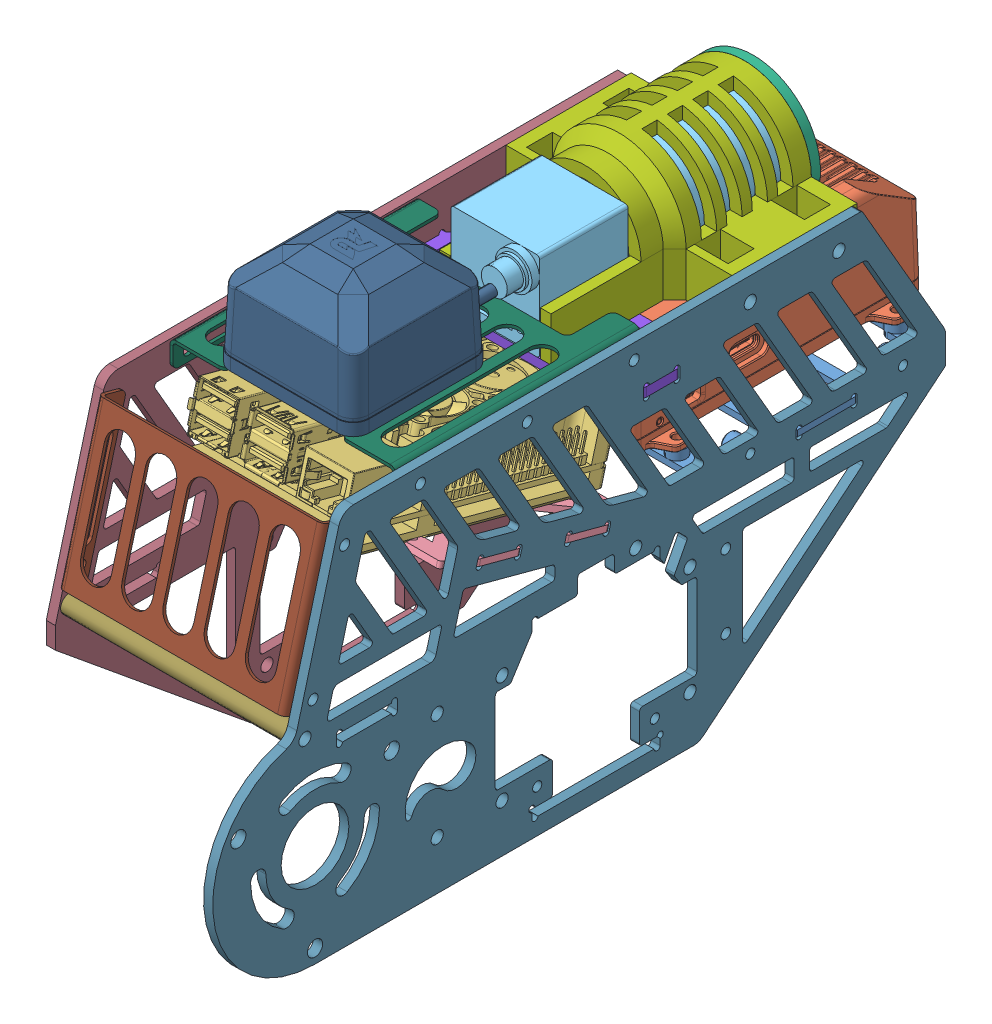
SolidWorks assembly pitch轴顶部设备, configuration 默认. Lengths in mm.
Overall size (80.14 158 249.05).
17 component instances, 15 part files, 47 mates.
Components (placement in the parent):
- 图传安装架-1: 图传安装架 [默认] at origin size (80 6 78)
- RM2019图传模块VT02-1: RM2019图传模块VT02 [默认] at (0 5 0.35) size (60 36.09 100.47)
- Raspberry Pi 4 Model B-1: Raspberry Pi 4 Model B [默认] at (0 22.2544 100.0052) x (0 0.258819 0.965926) z (-1 0 0) size (93.45 25.9 58.4)
- 树莓派安装板-1: 树莓派安装板 [默认] at (0 9.8234 92.9833) x (1 0 0) z (0 0.258819 0.965926) size (80 2 64)
- 相机MER-139-210U3C;HN-0612-2M-C1÷2X-1: 相机MER-139-210U3C;HN-0612-2M-C1÷2X [默认] at (0 53.5 39.5) x (0 1 0) z (1 0 0) size (32.45 89.5 29.5)
- 相机顶部保护PC板-1: 相机顶部保护PC板 [默认] at (0 53.5 -13) x (-1 0 0) z (0 0 -1) size (44 38.5 3)
- 相机顶部保护壳-1: 相机顶部保护壳 [默认] at (0 53.5 39) x (1 0 0) z (0 0 -1) size (74 36.5 81.5)
- 相机顶部安装板-1: 相机顶部安装板 [默认] at (0 36 39.5) size (80 3 29)
- hexagon socket head cap screws gb-1: hexagon socket head cap screws gb [GB_FASTENER_SCREWS_HSHCS M3X6-C] at (-10 33 41.8) x (0 1 0) z (0 0 -1) size (9 5.5 5.5)
- hexagon socket head cap screws gb-3: hexagon socket head cap screws gb [GB_FASTENER_SCREWS_HSHCS M3X6-C] at (10 33 41.8) x (0 1 0) z (0 0 -1) size (9 5.5 5.5)
- RM2019裁判系统定位模块UW01-1: RM2019裁判系统定位模块UW01 [默认] at (0 54 115) x (-1 0 0) z (0 0 -1) size (45.56 33.5 81.86)
- 后端钣金支撑-1: 后端钣金支撑 [默认] at (0 25.3462 167.3322) x (1 0 0) z (0 0.965926 -0.258819) size (74 9 50)
- 铝柱M4×74-定制-1: 铝柱M4×74-定制 [默认] at (37 -5 62.5) x (0 0 1) z (-1 0 0) size (6 6 74)
- 铝柱M4×74-定制-2: 铝柱M4×74-定制 [默认] at (37 -5 170.8047) x (0 0.986463 -0.163981) z (-1 0 0) size (6 6 74)
- pitch轴外框竖板-1: pitch轴外框竖板 [默认] at (-37 -37 75.5) x (-1 0 0) z (0 0 -1) size (3 124 214.5)
- pitch轴外框竖板-电机-1: pitch轴外框竖板-电机 [默认] at (40 -37 75.5) x (-1 0 0) z (0 0 -1) size (3.14 124 240)
- 顶部钣金支撑-1: 顶部钣金支撑 [默认] at (0 53 98) x (-1 0 0) z (0 0 1) size (74 9 80)
Mates (geometry in assembly coordinates):
- 重合4: coincident: plane of 图传安装架-1 through (-27 5 -36) normal (0 1 0); plane of RM2019图传模块VT02-1 through (-29.7 5 47.7) normal (0 -1 0)
- 同心1: concentric: cylinder of 图传安装架-1 through (-27 5 -36) axis (0 1 0) radius 1.025; cylinder of RM2019图传模块VT02-1 through (-27 5 -36) axis (0 1 0) radius 1.35
- 同心2: concentric: cylinder of 图传安装架-1 through (-27 5 36) axis (0 1 0) radius 1.025; cylinder of RM2019图传模块VT02-1 through (-27 6.7 36) axis (0 -1 0) radius 1.35
- 同心8: concentric: cylinder of Raspberry Pi 4 Model B-1 through (24.5 12.9332 62.1271) axis (0 0.965926 -0.258819) radius 1.35; cylinder of 树莓派安装板-1 through (24.5 4.2495 64.4538) axis (0 -0.965926 0.258819) radius 1.5
- 同心9: concentric: cylinder of Raspberry Pi 4 Model B-1 through (-24.5 12.9332 62.1271) axis (0 0.965926 -0.258819) radius 1.35; cylinder of 树莓派安装板-1 through (-24.5 4.2495 64.4538) axis (0 -0.965926 0.258819) radius 1.5
- 重合879: coincident: plane of Raspberry Pi 4 Model B-1 through (0 14.6023 103.0909) normal (0 -0.965926 0.258819); plane of 树莓派安装板-1 through (0 11.7553 92.4657) normal (0 0.965926 -0.258819)
- 同心52: concentric: cylinder of pitch轴外框竖板-1 through (-40 4.863 168.162) axis (1 0 0) radius 1.65; cylinder of 后端钣金支撑-1 through (-37 4.863 168.162) axis (1 0 0) radius 1.65
- 同心53: concentric: cylinder of pitch轴外框竖板-1 through (-40 43.5 157.8092) axis (1 0 0) radius 1.65; cylinder of 后端钣金支撑-1 through (-37 43.5 157.8092) axis (1 0 0) radius 1.65
- 重合48: coincident: plane of pitch轴外框竖板-1 through (-37 48.5 154.9165) normal (1 0 0); plane of 后端钣金支撑-1 through (-37 47.4238 153.1344) normal (-1 0 0)
- 同心60: concentric: cylinder of 相机MER-139-210U3C;HN-0612-2M-C1÷2X-1 through (-10 41.7 41.8) axis (0 -1 0) radius 1.25; cylinder of 相机顶部安装板-1 through (-10 39 41.8) axis (0 -1 0) radius 1.65
- 同心61: concentric: cylinder of 相机MER-139-210U3C;HN-0612-2M-C1÷2X-1 through (10 41.7 41.8) axis (0 -1 0) radius 1.25; cylinder of 相机顶部安装板-1 through (10 39 41.8) axis (0 -1 0) radius 1.65
- 重合52: coincident: plane of 相机MER-139-210U3C;HN-0612-2M-C1÷2X-1 through (14.5 39 68.5) normal (0 -1 0); plane of 相机顶部安装板-1 through (0 39 39.5) normal (0 1 0)
- 同心12: concentric: cylinder of 相机顶部安装板-1 through (-10 39 41.8) axis (0 -1 0) radius 1.65; cylinder of hexagon socket head cap screws gb-1 through (-10 42 41.8) axis (0 -1 0) radius 1.5
- 重合56: coincident: plane of 相机顶部安装板-1 through (0 36 39.5) normal (0 -1 0); plane of hexagon socket head cap screws gb-1 through (-10 36 41.8) normal (0 1 0)
- 同心14: concentric: cylinder of 相机顶部安装板-1 through (10 39 41.8) axis (0 -1 0) radius 1.65; cylinder of hexagon socket head cap screws gb-3 through (10 42 41.8) axis (0 -1 0) radius 1.5
- 重合6: coincident: plane of 相机顶部安装板-1 through (0 36 39.5) normal (0 -1 0); plane of hexagon socket head cap screws gb-3 through (10 36 41.8) normal (0 1 0)
- 距离3: distance = 4 mm: plane of RM2019图传模块VT02-1 through (-22.8755 30 46.8755) normal (0 1 0); plane of 相机顶部安装板-1 through (0 36 39.5) normal (0 -1 0)
- 重合66: coincident: plane of 图传安装架-1 through (-37 2 39) normal (-1 0 0); plane of pitch轴外框竖板-1 through (-37 48.5 154.9165) normal (1 0 0)
- 重合67: coincident: plane of 图传安装架-1 through (-40 2 39) normal (0 1 0); plane of pitch轴外框竖板-1 through (-40 2 -10) normal (0 -1 0)
- 重合68: coincident: plane of 图传安装架-1 through (-40 0 -10) normal (0 0 -1); plane of pitch轴外框竖板-1 through (-40 0 -10) normal (0 0 1)
- 重合69: coincident: plane of 树莓派安装板-1 through (0 11.7553 92.4657) normal (0 0.965926 -0.258819); plane of pitch轴外框竖板-1 through (-37 13.6964 99.7101) normal (0 -0.965926 0.258819)
- 重合70: coincident: plane of 树莓派安装板-1 through (-37 13.6964 99.7101) normal (0 -0.258819 -0.965926); plane of pitch轴外框竖板-1 through (-37 11.7646 100.2278) normal (0 0.258819 0.965926)
- 重合71: coincident: plane of 树莓派安装板-1 through (-37 9.8141 85.2212) normal (-1 0 0); plane of pitch轴外框竖板-1 through (-37 48.5 154.9165) normal (1 0 0)
- 重合72: coincident: plane of 相机顶部安装板-1 through (0 39 39.5) normal (0 1 0); plane of pitch轴外框竖板-1 through (-37 39 60) normal (0 -1 0)
- 重合73: coincident: plane of 相机顶部安装板-1 through (-40 39 48) normal (0 0 -1); plane of pitch轴外框竖板-1 through (-37 39 48) normal (0 0 1)
- 重合74: coincident: plane of 相机顶部安装板-1 through (-37 39 48) normal (-1 0 0); plane of pitch轴外框竖板-1 through (-37 48.5 154.9165) normal (1 0 0)
- 同心86: concentric: cylinder of pitch轴外框竖板-1 through (-40 -5 62.5) axis (1 0 0) radius 2; cylinder of 铝柱M4×74-定制-1 through (-37 -5 62.5) axis (-1 0 0) radius 1.65
- 重合75: coincident: plane of pitch轴外框竖板-1 through (-37 48.5 154.9165) normal (1 0 0); plane of 铝柱M4×74-定制-1 through (-37 -5 62.5) normal (-1 0 0)
- 同心88: concentric: cylinder of pitch轴外框竖板-1 through (-40 -5 170.8047) axis (1 0 0) radius 2; cylinder of 铝柱M4×74-定制-2 through (-37 -5 170.8047) axis (-1 0 0) radius 1.65
- 重合77: coincident: plane of pitch轴外框竖板-1 through (-37 48.5 154.9165) normal (1 0 0); plane of 铝柱M4×74-定制-2 through (-37 -5 170.8047) normal (-1 0 0)
- 同心89: concentric: cylinder of 相机顶部保护PC板-1 through (0 53.5 -16) axis (0 0 1) radius 22; cylinder of 相机顶部保护壳-1 through (0 53.5 47.4743) axis (0 0 1) radius 16
- 同心90: concentric: cylinder of 相机MER-139-210U3C;HN-0612-2M-C1÷2X-1 through (0 53.5 24.5) axis (0 0 1) radius 14; cylinder of 相机顶部保护壳-1 through (0 53.5 47.4743) axis (0 0 1) radius 14.25
- 距离4: distance = 0.5 mm: plane of 相机顶部保护壳-1 through (14.25 53.5 25) normal (0 0 -1); plane of 相机MER-139-210U3C;HN-0612-2M-C1÷2X-1 through (0 53.5 24.5) normal (0 0 1)
- 重合79: coincident: plane of 相机顶部安装板-1 through (0 39 39.5) normal (0 1 0); plane of 相机顶部保护壳-1 through (0 39 39) normal (0 -1 0)
- 重合80: coincident: plane of 相机顶部保护PC板-1 through (0 53.5 -13) normal (0 0 1); plane of 相机顶部保护壳-1 through (0 53.5 -13) normal (0 0 -1)
- 同心91: concentric: cylinder of 相机顶部保护PC板-1 through (19 53.5 -16) axis (0 0 1) radius 1.5; cylinder of 相机顶部保护壳-1 through (19 53.5 -13) axis (0 0 -1) radius 1.25
- 同心93: concentric: cylinder of 图传安装架-1 through (37 3 -25) axis (1 0 0) radius 1.25; cylinder of pitch轴外框竖板-电机-1 through (37 3 -25) axis (1 0 0) radius 1.5
- 同心94: concentric: cylinder of 图传安装架-1 through (37 3 25) axis (1 0 0) radius 1.25; cylinder of pitch轴外框竖板-电机-1 through (37 3 25) axis (1 0 0) radius 1.5
- 重合84: coincident: plane of 图传安装架-1 through (37 2 39) normal (1 0 0); plane of pitch轴外框竖板-电机-1 through (37 48.5 154.9165) normal (-1 0 0)
- 同心95: concentric: cylinder of pitch轴外框竖板-1 through (-40 48.5 133) axis (1 0 0) radius 1.65; cylinder of 顶部钣金支撑-1 through (37 48.5 133) axis (-1 0 0) radius 1.65
- 重合85: coincident: plane of pitch轴外框竖板-1 through (-37 48.5 154.9165) normal (1 0 0); plane of 顶部钣金支撑-1 through (-37 53 138) normal (-1 0 0)
- 同心96: concentric: cylinder of pitch轴外框竖板-1 through (-40 48.5 63) axis (1 0 0) radius 1.65; cylinder of 顶部钣金支撑-1 through (37 48.5 63) axis (-1 0 0) radius 1.65
- 重合86: coincident: plane of RM2019裁判系统定位模块UW01-1 through (22.75 54 92.25) normal (0 -1 0); plane of 顶部钣金支撑-1 through (36 54 138) normal (0 1 0)
- 同心97: concentric: cylinder of RM2019裁判系统定位模块UW01-1 through (19 58.5 115) axis (0 -1 0) radius 1.25; cylinder of 顶部钣金支撑-1 through (19 53 115) axis (0 1 0) radius 1.5
- 同心98: concentric: cylinder of RM2019裁判系统定位模块UW01-1 through (-19 58.5 115) axis (0 -1 0) radius 1.25; cylinder of 顶部钣金支撑-1 through (-19 53 115) axis (0 1 0) radius 1.5
- 同心1065: concentric: cylinder of pitch轴外框竖板-1 through (-40 46 -4) axis (1 0 0) radius 2; cylinder of ? through (-28 46 -4) axis (-1 0 0) radius 2
- 重合93: coincident: plane of pitch轴外框竖板-1 through (-40 48.5 154.9165) normal (-1 0 0); plane of ? through (-40 46 -4) normal (1 0 0)
